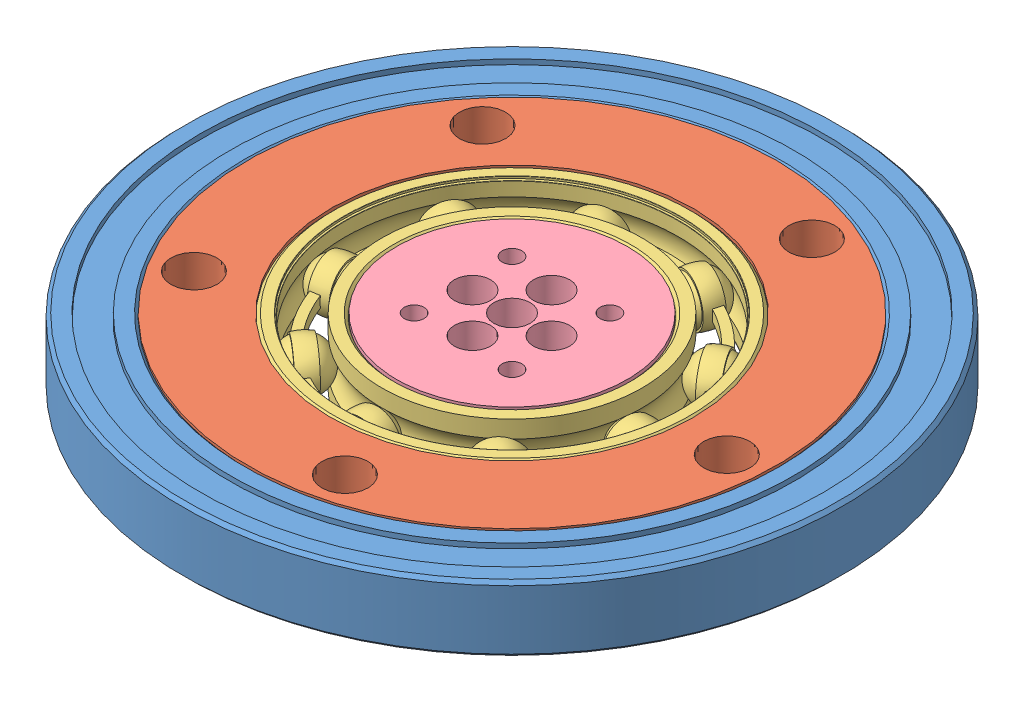
SolidWorks assembly Center Cap, configuration Default. Lengths in mm.
Overall size (111.74 25 111.74).
4 component instances, 4 part files, 6 mates.
Components (placement in the parent):
- 6656K245_Ultra-Thin Ball Bearing-1: 6656K245_Ultra-Thin Ball Bearing [6656K245] at (42.001 57.7314 86.0053) x (0.992128 0 0.125231) z (0 1 0) size (100 100 10)
- Bearing Ring-1: Bearing Ring [Default] at (42.001 62.7314 86.0053) x (0.532714 0 0.846296) z (0.846296 0 -0.532714) size (80.25 10 80.25)
- 5972K248_Ball Bearing-1: 5972K248_Ball Bearing [5972K248] at (42.001 57.7314 86.0053) x (-0.523528 0 -0.852009) z (0 -1 0) size (55 55 10)
- Input Shaft-1: Input Shaft [end] at (42.001 17.7314 86.0053) size (37.5 25 37.5)
Mates (geometry in assembly coordinates):
- Concentric1: concentric aligned: cylinder of 6656K245_Ultra-Thin Ball Bearing-1 through (42.001 62.7314 86.0053) axis (0 1 0) radius 40; cylinder of Bearing Ring-1 through (42.001 52.7314 86.0053) axis (0 1 0) radius 40.125
- Coincident1: coincident aligned: plane of 6656K245_Ultra-Thin Ball Bearing-1 through (47.0729 52.7314 45.8241) normal (0 -1 0); plane of Bearing Ring-1 through (42.001 52.7314 86.0053) normal (0 -1 0)
- Concentric2: concentric aligned: cylinder of Bearing Ring-1 through (42.001 62.7314 86.0053) axis (0 -1 0) radius 27.5; cylinder of 5972K248_Ball Bearing-1 through (42.001 52.7314 86.0053) axis (0 -1 0) radius 17.4995
- Coincident2: coincident aligned: plane of Bearing Ring-1 through (42.001 52.7314 86.0053) normal (0 -1 0); circle of 5972K248_Ball Bearing-1
- Concentric3: concentric aligned: cylinder of 5972K248_Ball Bearing-1 through (42.001 52.7314 86.0053) axis (0 -1 0) radius 17.4995; cylinder of Input Shaft-1 through (42.001 62.7314 86.0053) axis (0 -1 0) radius 17.5
- Coincident3: coincident aligned: plane of Bearing Ring-1 through (42.001 62.7314 86.0053) normal (0 1 0); plane of Input Shaft-1 through (42.001 62.7314 86.0053) normal (0 1 0)
